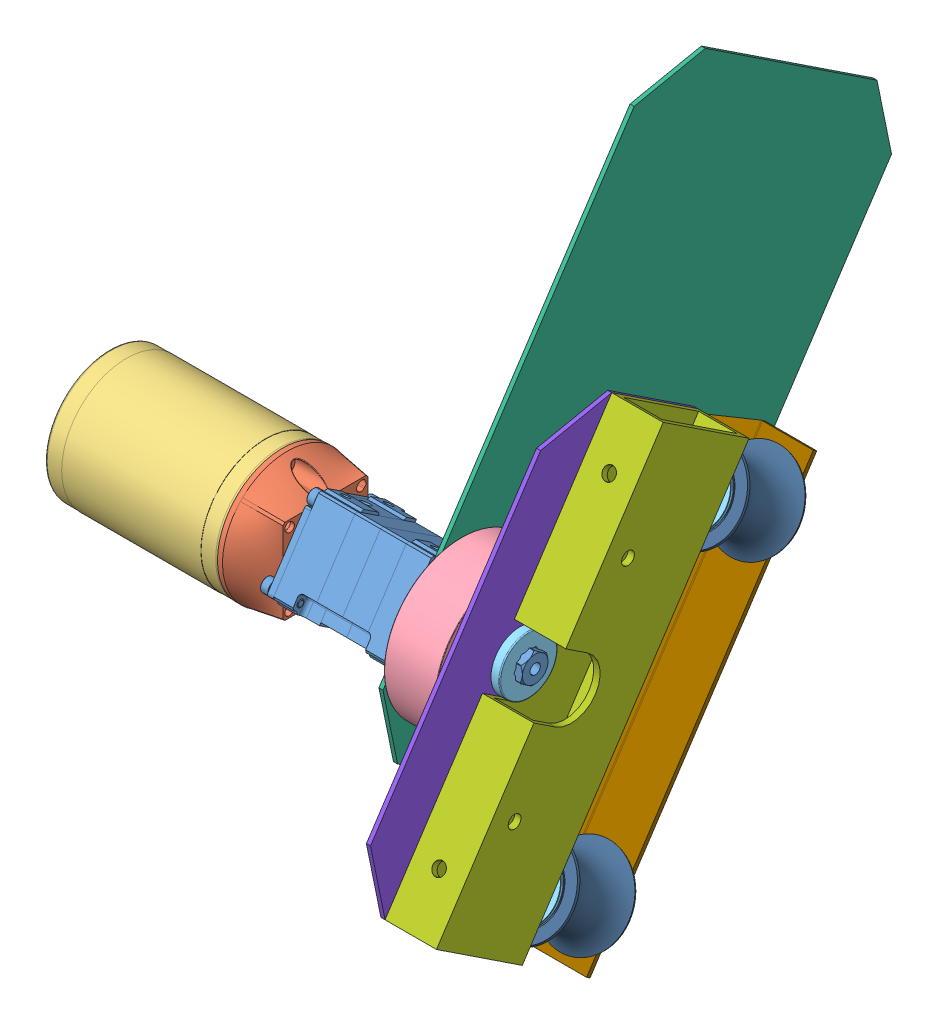
SolidWorks assembly ClimberWithoutPipe, configuration Default. Lengths in mm.
Overall size (242.1 332.1 318.45).
16 component instances, 10 part files, 0 mates.
Components (placement in the parent):
- ClimberWithoutPipe.stp-1: ClimberWithoutPipe.stp [Default] at origin size (242.1 332.1 318.45)
  - VersaPlanetary_v2_Two_Stage_100_1_with_BAG.stp-1: VersaPlanetary_v2_Two_Stage_100_1_with_BAG.stp [Default] at (-147.4647 -756.6918 -846.1082) x (1 0 0) z (0 0.551291 0.834313) size (110.6 44.45 42.65)
  - VersaPlanetary_CIM_Adapter_217-4018.stp-1: VersaPlanetary_CIM_Adapter_217-4018.stp [Default] at (-203.6897 -738.1492 -858.3607) x (0 -1 0) z (0 0 1) size (64.01 21.55 64.01)
  - Mini_CIM_Motor_217-3371.stp-1: Mini_CIM_Motor_217-3371.stp [Default] at (-215.2147 -738.1492 -858.3607) x (-1 0 0) z (0 0.447307 -0.894381) size (125.82 64.01 64.01)
  - am-3945 3IN 500Hex Compliant Wheel VER 3.stp-1: am-3945 3IN 500Hex Compliant Wheel VER 3.stp [Default] at (-85.5106 -746.8798 -917.1009) x (0 -0.212917 -0.97707) z (-1 0 0) size (76.2 76.2 25.4)
  - am-2986 FR8ZZ Hex Bearing.stp-1: am-2986 FR8ZZ Hex Bearing.stp [Default] at (-93.4483 -738.1492 -858.3607) x (0 0 1) z (-1 0 0) size (31.12 31.12 7.93)
  - Bottom Wheel Plate.stp-1: Bottom Wheel Plate.stp [Default] at (-130.8397 -707.3598 -852.079) x (0 0.834313 -0.551291) z (1 0 0) size (275.87 152.4 2.03)
  - Top Bar.stp-1: Top Bar.stp [Default] at (-97.8197 -794.7225 -805.7565) x (0 -0.551291 -0.834313) z (1 0 0) size (50.8 203.2 25.4)
  - Top Wheel Plate.stp-1: Top Wheel Plate.stp [Default] at (-97.8197 -745.1506 -868.9565) x (0 0.551291 0.834313) z (-1 0 0) size (76.2 203.2 2.03)
  - am-2986 FR8ZZ Hex Bearing.stp-2: am-2986 FR8ZZ Hex Bearing.stp [Default] at (-85.1197 -827.0983 -854.7535) x (1 0 0) z (0 0.551291 0.834313) size (31.12 31.12 7.93)
  - am-2986 FR8ZZ Hex Bearing.stp-3: am-2986 FR8ZZ Hex Bearing.stp [Default] at (-85.1197 -699.949 -938.7703) x (1 0 0) z (0 0.551291 0.834313) size (31.12 31.12 7.93)
  - am-2986 FR8ZZ Hex Bearing.stp-4: am-2986 FR8ZZ Hex Bearing.stp [Default] at (-85.1197 -839.362 -873.3131) x (1 0 0) z (0 -0.551291 -0.834313) size (31.12 31.12 7.93)
  - am-2986 FR8ZZ Hex Bearing.stp-5: am-2986 FR8ZZ Hex Bearing.stp [Default] at (-85.1197 -712.2126 -957.3298) x (1 0 0) z (0 -0.551291 -0.834313) size (31.12 31.12 7.93)
  - Side Plate.stp-1: Side Plate.stp [Default] at (-69.5622 -843.7322 -879.927) x (1 0 0) z (0 -0.551291 -0.834313) size (100.44 203.2 15.23)
  - Roller.stp-1: Roller.stp [Default] at (-85.1197 -827.0983 -854.7535) x (-1 0 0) z (0 -0.551291 -0.834313) size (43.57 43.57 34.54)
  - Roller.stp-2: Roller.stp [Default] at (-85.1197 -699.949 -938.7703) x (-1 0 0) z (0 -0.551291 -0.834313) size (43.57 43.57 34.54)
